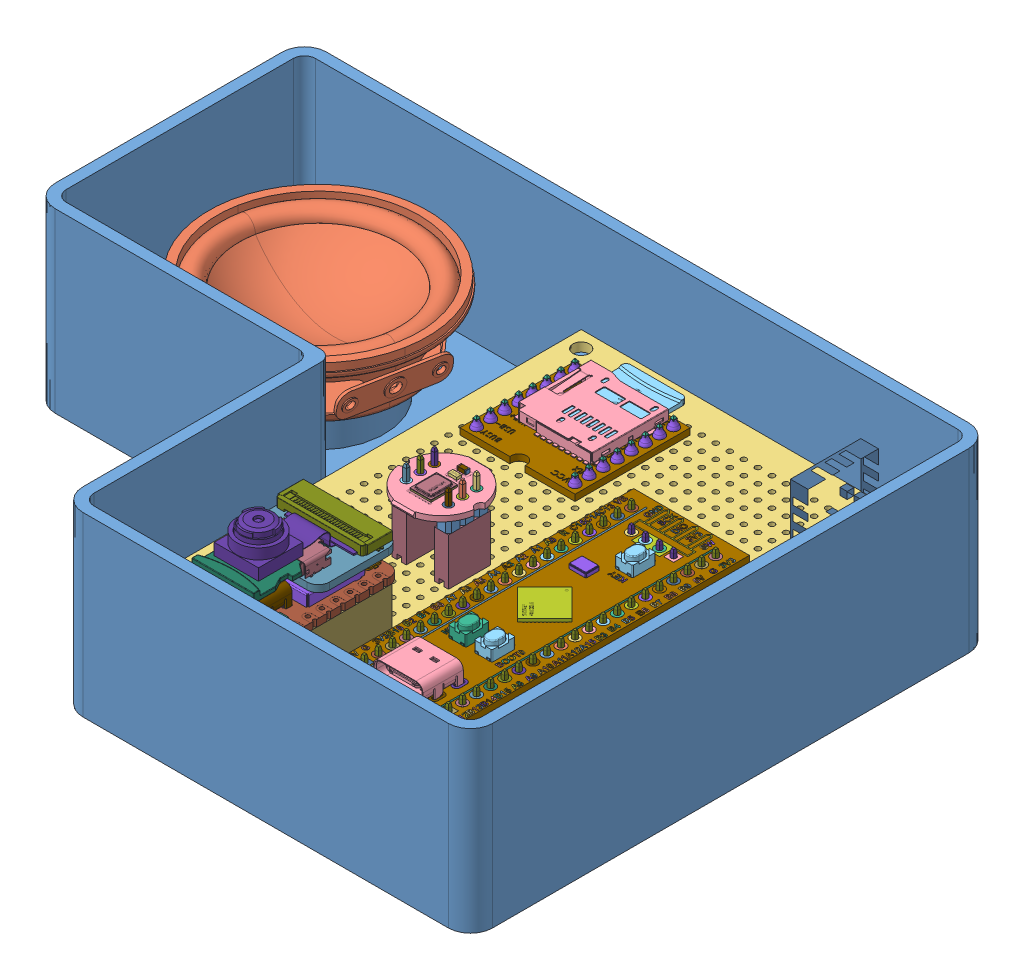
SolidWorks assembly FullLapRapVoHop, configuration Default. Lengths in mm.
Overall size (124 38.8 94).
334 component instances, 247 part files, 6 mates.
Components (placement in the parent):
- DeHop7x9-1: DeHop7x9 [Default] at (43.7132 25.4201 123.2311) size (124 32 94)
- SPEAKER 4OHM 3W.step-1: SPEAKER 4OHM 3W.step [Default] at (18.7132 43.1201 55.7311) x (-0.187693 0 0.982228) z (0.982228 0 0.187693) size (40 18.1 40)
- 3D_Final-2: 3D_Final [Default] at (43.7132 35.4201 33.2311) size (70 34.34 90)
  - BoardDong7x9-1: BoardDong7x9 [Default] at (35 1.6 45) x (0 0 -1) z (0 1 0) size (90 70 2.6)
  - blackpill v2.0 swi.STEP-1: blackpill v2.0 swi.STEP [Default] at (52.8 12.64 59.37) x (0 0 -1) z (0 1 0) size (53 20.9 10.45)
    - blackpill v2.0.step.STEP-1: blackpill v2.0.step.STEP [Default] at origin size (53 20.9 4.92)
      - USB Type C Port (SMD Type).step.STEP-1: USB Type C Port (SMD Type).step.STEP [Default] at (-19.2 0 3.305) x (0 -1 0) z (0 0 -1) size (8.94 7.9 4.2)
      - PTS810 SJK 250 SMTR LFS--3DModel-STEP-1.step.STEP-1: PTS810 SJK 250 SMTR LFS--3DModel-STEP-1.step.STEP [Default] at (14.5 -1.8498 1.7) x (1 0 0) z (0 -1 0) size (4.6 2.51 3.2)
      - PTS810 SJK 250 SMTR LFS--3DModel-STEP-1.step.STEP-2: PTS810 SJK 250 SMTR LFS--3DModel-STEP-1.step.STEP [Default] at (-11.4 -2.3498 1.7) x (1 0 0) z (0 -1 0) size (4.6 2.51 3.2)
      - PTS810 SJK 250 SMTR LFS--3DModel-STEP-1 v2(Mirror).step.STEP-1: PTS810 SJK 250 SMTR LFS--3DModel-STEP-1 v2(Mirror).step.STEP [Default] at (-11.4 2.3498 1.7) x (1 0 0) z (0 -1 0) size (4.6 2.51 3.2)
      - STM32F411CEU6.step.STEP-1: STM32F411CEU6.step.STEP [Default] at (0 0 1.7) x (-0.707107 -0.707107 0) z (-0.707107 0.707107 0) size (7 0.6 7)
      - ECS-135.60-12-33Q-JES-TR.step.STEP-1: ECS-135.60-12-33Q-JES-TR.step.STEP [Default] at (9.3867 2.3215 1.7) x (0 -1 0) z (-1 0 0) size (3.2 0.8 2.5)
      - DIY_black_pill.step.STEP-1: DIY_black_pill.step.STEP [Default] at origin size (53 20.9 1.7)
      - DIY_black_pill-0.step.STEP-1: DIY_black_pill-0.step.STEP [Default] at origin size (1.8 1.8 1.72)
      - DIY_black_pill-1.step.STEP-1: DIY_black_pill-1.step.STEP [Default] at origin size (1.8 1.8 1.72)
      - DIY_black_pill-2.step.STEP-1: DIY_black_pill-2.step.STEP [Default] at origin size (1.8 1.8 1.72)
      - DIY_black_pill-3.step.STEP-1: DIY_black_pill-3.step.STEP [Default] at origin size (1.8 1.8 1.72)
      - DIY_black_pill-4.step.STEP-1: DIY_black_pill-4.step.STEP [Default] at origin size (1.8 1.8 1.72)
      - DIY_black_pill-5.step.STEP-1: DIY_black_pill-5.step.STEP [Default] at origin size (1.8 1.8 1.72)
      - DIY_black_pill-6.step.STEP-1: DIY_black_pill-6.step.STEP [Default] at origin size (1.8 1.8 1.72)
      - DIY_black_pill-7.step.STEP-1: DIY_black_pill-7.step.STEP [Default] at origin size (1.8 1.8 1.72)
      - DIY_black_pill-8.step.STEP-1: DIY_black_pill-8.step.STEP [Default] at origin size (1.8 1.8 1.72)
      - DIY_black_pill-9.step.STEP-1: DIY_black_pill-9.step.STEP [Default] at origin size (1.8 1.8 1.72)
      - DIY_black_pill-10.step.STEP-1: DIY_black_pill-10.step.STEP [Default] at origin size (1.8 1.8 1.72)
      - DIY_black_pill-11.step.STEP-1: DIY_black_pill-11.step.STEP [Default] at origin size (1.8 1.8 1.72)
      - DIY_black_pill-12.step.STEP-1: DIY_black_pill-12.step.STEP [Default] at origin size (1.8 1.8 1.72)
      - DIY_black_pill-13.step.STEP-1: DIY_black_pill-13.step.STEP [Default] at origin size (1.8 1.8 1.72)
      - DIY_black_pill-14.step.STEP-1: DIY_black_pill-14.step.STEP [Default] at origin size (1.8 1.8 1.72)
      - DIY_black_pill-15.step.STEP-1: DIY_black_pill-15.step.STEP [Default] at origin size (1.8 1.8 1.72)
      - DIY_black_pill-16.step.STEP-1: DIY_black_pill-16.step.STEP [Default] at origin size (1.8 1.8 1.72)
      - DIY_black_pill-17.step.STEP-1: DIY_black_pill-17.step.STEP [Default] at origin size (1.8 1.8 1.72)
      - DIY_black_pill-18.step.STEP-1: DIY_black_pill-18.step.STEP [Default] at origin size (1.8 1.8 1.72)
      - DIY_black_pill-19.step.STEP-1: DIY_black_pill-19.step.STEP [Default] at origin size (1.8 1.8 1.72)
      - DIY_black_pill-20.step.STEP-1: DIY_black_pill-20.step.STEP [Default] at origin size (1.8 1.8 1.72)
      - DIY_black_pill-21.step.STEP-1: DIY_black_pill-21.step.STEP [Default] at origin size (1.8 1.8 1.72)
      - DIY_black_pill-22.step.STEP-1: DIY_black_pill-22.step.STEP [Default] at origin size (1.8 1.8 1.72)
      - DIY_black_pill-23.step.STEP-1: DIY_black_pill-23.step.STEP [Default] at origin size (1.8 1.8 1.72)
      - DIY_black_pill-24.step.STEP-1: DIY_black_pill-24.step.STEP [Default] at origin size (1.8 1.8 1.72)
      - DIY_black_pill-25.step.STEP-1: DIY_black_pill-25.step.STEP [Default] at origin size (1.8 1.8 1.72)
      - DIY_black_pill-26.step.STEP-1: DIY_black_pill-26.step.STEP [Default] at origin size (1.8 1.8 1.72)
      - DIY_black_pill-27.step.STEP-1: DIY_black_pill-27.step.STEP [Default] at origin size (1.8 1.8 1.72)
      - DIY_black_pill-28.step.STEP-1: DIY_black_pill-28.step.STEP [Default] at origin size (1.8 1.8 1.72)
      - DIY_black_pill-29.step.STEP-1: DIY_black_pill-29.step.STEP [Default] at origin size (1.8 1.8 1.72)
      - DIY_black_pill-30.step.STEP-1: DIY_black_pill-30.step.STEP [Default] at origin size (1.8 1.8 1.72)
      - DIY_black_pill-31.step.STEP-1: DIY_black_pill-31.step.STEP [Default] at origin size (1.8 1.8 1.72)
      - DIY_black_pill-32.step.STEP-1: DIY_black_pill-32.step.STEP [Default] at origin size (1.8 1.8 1.72)
      - DIY_black_pill-33.step.STEP-1: DIY_black_pill-33.step.STEP [Default] at origin size (1.8 1.8 1.72)
      - DIY_black_pill-34.step.STEP-1: DIY_black_pill-34.step.STEP [Default] at origin size (1.8 1.8 1.72)
      - DIY_black_pill-35.step.STEP-1: DIY_black_pill-35.step.STEP [Default] at origin size (1.8 1.8 1.72)
      - DIY_black_pill-36.step.STEP-1: DIY_black_pill-36.step.STEP [Default] at origin size (1.8 1.8 1.72)
      - DIY_black_pill-37.step.STEP-1: DIY_black_pill-37.step.STEP [Default] at origin size (1.8 1.8 1.72)
      - DIY_black_pill-38.step.STEP-1: DIY_black_pill-38.step.STEP [Default] at origin size (1.8 1.8 1.72)
      - DIY_black_pill-39.step.STEP-1: DIY_black_pill-39.step.STEP [Default] at origin size (1.8 1.8 1.72)
      - DIY_black_pill-40.step.STEP-1: DIY_black_pill-40.step.STEP [Default] at origin size (51.2 0.3 0.01)
      - DIY_black_pill-41.step.STEP-1: DIY_black_pill-41.step.STEP [Default] at origin size (51.2 0.3 0.01)
      - DIY_black_pill-42.step.STEP-1: DIY_black_pill-42.step.STEP [Default] at origin size (0.93 1 0.01)
      - DIY_black_pill-43.step.STEP-1: DIY_black_pill-43.step.STEP [Default] at origin size (0.94 1.03 0.01)
      - DIY_black_pill-44.step.STEP-1: DIY_black_pill-44.step.STEP [Default] at origin size (0.93 1 0.01)
      - DIY_black_pill-45.step.STEP-1: DIY_black_pill-45.step.STEP [Default] at origin size (0.67 1.02 0.01)
      - DIY_black_pill-46.step.STEP-1: DIY_black_pill-46.step.STEP [Default] at origin size (0.66 1.02 0.01)
      - DIY_black_pill-47.step.STEP-1: DIY_black_pill-47.step.STEP [Default] at origin size (0.84 1 0.01)
      - DIY_black_pill-48.step.STEP-1: DIY_black_pill-48.step.STEP [Default] at origin size (0.67 1.02 0.01)
      - DIY_black_pill-49.step.STEP-1: DIY_black_pill-49.step.STEP [Default] at origin size (0.84 1.01 0.01)
      - DIY_black_pill-50.step.STEP-1: DIY_black_pill-50.step.STEP [Default] at origin size (0.72 1.01 0.01)
      - DIY_black_pill-51.step.STEP-1: DIY_black_pill-51.step.STEP [Default] at origin size (0.84 1 0.01)
      - DIY_black_pill-52.step.STEP-1: DIY_black_pill-52.step.STEP [Default] at origin size (0.67 1 0.01)
      - DIY_black_pill-53.step.STEP-1: DIY_black_pill-53.step.STEP [Default] at origin size (1 1 0.01)
      - DIY_black_pill-54.step.STEP-1: DIY_black_pill-54.step.STEP [Default] at origin size (0.44 1 0.01)
      - DIY_black_pill-55.step.STEP-1: DIY_black_pill-55.step.STEP [Default] at origin size (0.44 1 0.01)
      - DIY_black_pill-56.step.STEP-1: DIY_black_pill-56.step.STEP [Default] at origin size (1 1 0.01)
      - DIY_black_pill-57.step.STEP-1: DIY_black_pill-57.step.STEP [Default] at origin size (0.44 1 0.01)
      - DIY_black_pill-58.step.STEP-1: DIY_black_pill-58.step.STEP [Default] at origin size (0.67 1.02 0.01)
      - DIY_black_pill-59.step.STEP-1: DIY_black_pill-59.step.STEP [Default] at origin size (0.66 1.02 0.01)
      - DIY_black_pill-60.step.STEP-1: DIY_black_pill-60.step.STEP [Default] at origin size (0.67 1 0.01)
      - DIY_black_pill-61.step.STEP-1: DIY_black_pill-61.step.STEP [Default] at origin size (0.84 1 0.01)
      - DIY_black_pill-62.step.STEP-1: DIY_black_pill-62.step.STEP [Default] at origin size (0.44 1 0.01)
      - DIY_black_pill-63.step.STEP-1: DIY_black_pill-63.step.STEP [Default] at origin size (0.66 1.02 0.01)
      - DIY_black_pill-64.step.STEP-1: DIY_black_pill-64.step.STEP [Default] at origin size (0.44 1 0.01)
      - DIY_black_pill-65.step.STEP-1: DIY_black_pill-65.step.STEP [Default] at origin size (0.84 1 0.01)
      - DIY_black_pill-66.step.STEP-1: DIY_black_pill-66.step.STEP [Default] at origin size (0.72 1 0.01)
      - DIY_black_pill-67.step.STEP-1: DIY_black_pill-67.step.STEP [Default] at origin size (0.44 1 0.01)
      - DIY_black_pill-68.step.STEP-1: DIY_black_pill-68.step.STEP [Default] at origin size (0.84 1 0.01)
      - DIY_black_pill-69.step.STEP-1: DIY_black_pill-69.step.STEP [Default] at origin size (1 1 0.01)
      - DIY_black_pill-70.step.STEP-1: DIY_black_pill-70.step.STEP [Default] at origin size (1 1 0.01)
      - DIY_black_pill-71.step.STEP-1: DIY_black_pill-71.step.STEP [Default] at origin size (0.65 1.02 0.01)
      - DIY_black_pill-72.step.STEP-1: DIY_black_pill-72.step.STEP [Default] at origin size (0.44 1 0.01)
      - DIY_black_pill-73.step.STEP-1: DIY_black_pill-73.step.STEP [Default] at origin size (1 1 0.01)
      - DIY_black_pill-74.step.STEP-1: DIY_black_pill-74.step.STEP [Default] at origin size (0.67 1 0.01)
      - DIY_black_pill-75.step.STEP-1: DIY_black_pill-75.step.STEP [Default] at origin size (0.44 1 0.01)
      - DIY_black_pill-76.step.STEP-1: DIY_black_pill-76.step.STEP [Default] at origin size (1 1 0.01)
      - DIY_black_pill-77.step.STEP-1: DIY_black_pill-77.step.STEP [Default] at origin size (0.66 1.02 0.01)
      - DIY_black_pill-78.step.STEP-1: DIY_black_pill-78.step.STEP [Default] at origin size (0.84 1.01 0.01)
      - DIY_black_pill-79.step.STEP-1: DIY_black_pill-79.step.STEP [Default] at origin size (0.67 1.01 0.01)
      - DIY_black_pill-80.step.STEP-1: DIY_black_pill-80.step.STEP [Default] at origin size (0.84 1 0.01)
      - DIY_black_pill-81.step.STEP-1: DIY_black_pill-81.step.STEP [Default] at origin size (0.66 0.99 0.01)
      - DIY_black_pill-82.step.STEP-1: DIY_black_pill-82.step.STEP [Default] at origin size (0.84 1 0.01)
      - DIY_black_pill-83.step.STEP-1: DIY_black_pill-83.step.STEP [Default] at origin size (0.84 1 0.01)
      - DIY_black_pill-84.step.STEP-1: DIY_black_pill-84.step.STEP [Default] at origin size (0.67 1 0.01)
      - DIY_black_pill-85.step.STEP-1: DIY_black_pill-85.step.STEP [Default] at origin size (0.66 1.02 0.01)
      - DIY_black_pill-86.step.STEP-1: DIY_black_pill-86.step.STEP [Default] at origin size (0.66 1.02 0.01)
      - DIY_black_pill-87.step.STEP-1: DIY_black_pill-87.step.STEP [Default] at origin size (0.67 1 0.01)
      - DIY_black_pill-88.step.STEP-1: DIY_black_pill-88.step.STEP [Default] at origin size (0.44 1 0.01)
      - DIY_black_pill-89.step.STEP-1: DIY_black_pill-89.step.STEP [Default] at origin size (0.84 1 0.01)
      - DIY_black_pill-90.step.STEP-1: DIY_black_pill-90.step.STEP [Default] at origin size (1 1 0.01)
      - DIY_black_pill-91.step.STEP-1: DIY_black_pill-91.step.STEP [Default] at origin size (0.84 1 0.01)
      - DIY_black_pill-92.step.STEP-1: DIY_black_pill-92.step.STEP [Default] at origin size (0.44 1 0.01)
      - DIY_black_pill-93.step.STEP-1: DIY_black_pill-93.step.STEP [Default] at origin size (0.87 1.03 0.01)
      - DIY_black_pill-94.step.STEP-1: DIY_black_pill-94.step.STEP [Default] at origin size (0.44 1 0.01)
      - DIY_black_pill-95.step.STEP-1: DIY_black_pill-95.step.STEP [Default] at origin size (0.44 1 0.01)
      - DIY_black_pill-96.step.STEP-1: DIY_black_pill-96.step.STEP [Default] at origin size (0.9 1 0.01)
      - DIY_black_pill-97.step.STEP-1: DIY_black_pill-97.step.STEP [Default] at origin size (0.65 1.02 0.01)
      - DIY_black_pill-98.step.STEP-1: DIY_black_pill-98.step.STEP [Default] at origin size (1 1 0.01)
      - DIY_black_pill-99.step.STEP-1: DIY_black_pill-99.step.STEP [Default] at origin size (0.72 1 0.01)
      - DIY_black_pill-100.step.STEP-1: DIY_black_pill-100.step.STEP [Default] at origin size (1 1 0.01)
      - DIY_black_pill-101.step.STEP-1: DIY_black_pill-101.step.STEP [Default] at origin size (0.67 1.02 0.01)
      - DIY_black_pill-102.step.STEP-1: DIY_black_pill-102.step.STEP [Default] at origin size (0.65 1.02 0.01)
      - DIY_black_pill-103.step.STEP-1: DIY_black_pill-103.step.STEP [Default] at origin size (1 1 0.01)
      - DIY_black_pill-104.step.STEP-1: DIY_black_pill-104.step.STEP [Default] at origin size (0.84 1 0.01)
      - DIY_black_pill-105.step.STEP-1: DIY_black_pill-105.step.STEP [Default] at origin size (0.84 1 0.01)
      - DIY_black_pill-106.step.STEP-1: DIY_black_pill-106.step.STEP [Default] at origin size (0.65 1.02 0.01)
      - DIY_black_pill-107.step.STEP-1: DIY_black_pill-107.step.STEP [Default] at origin size (0.66 1.02 0.01)
      - DIY_black_pill-108.step.STEP-1: DIY_black_pill-108.step.STEP [Default] at origin size (0.66 1.02 0.01)
      - DIY_black_pill-109.step.STEP-1: DIY_black_pill-109.step.STEP [Default] at origin size (0.67 1 0.01)
      - DIY_black_pill-110.step.STEP-1: DIY_black_pill-110.step.STEP [Default] at origin size (0.93 1 0.01)
      - DIY_black_pill-111.step.STEP-1: DIY_black_pill-111.step.STEP [Default] at origin size (0.94 1.03 0.01)
      - DIY_black_pill-112.step.STEP-1: DIY_black_pill-112.step.STEP [Default] at origin size (0.93 1 0.01)
      - DIY_black_pill-113.step.STEP-1: DIY_black_pill-113.step.STEP [Default] at origin size (0.44 1 0.01)
      - DIY_black_pill-114.step.STEP-1: DIY_black_pill-114.step.STEP [Default] at origin size (0.84 1 0.01)
      - DIY_black_pill-115.step.STEP-1: DIY_black_pill-115.step.STEP [Default] at origin size (0.67 1 0.01)
      - DIY_black_pill-116.step.STEP-1: DIY_black_pill-116.step.STEP [Default] at origin size (0.44 1 0.01)
      - DIY_black_pill-117.step.STEP-1: DIY_black_pill-117.step.STEP [Default] at origin size (0.66 0.99 0.01)
      - DIY_black_pill-118.step.STEP-1: DIY_black_pill-118.step.STEP [Default] at origin size (0.84 1 0.01)
      - DIY_black_pill-119.step.STEP-1: DIY_black_pill-119.step.STEP [Default] at origin size (1 1 0.01)
      - DIY_black_pill-120.step.STEP-1: DIY_black_pill-120.step.STEP [Default] at origin size (0.67 1 0.01)
      - DIY_black_pill-121.step.STEP-1: DIY_black_pill-121.step.STEP [Default] at origin size (1 1 0.01)
      - DIY_black_pill-122.step.STEP-1: DIY_black_pill-122.step.STEP [Default] at origin size (0.66 1.02 0.01)
      - DIY_black_pill-123.step.STEP-1: DIY_black_pill-123.step.STEP [Default] at origin size (1 1 0.01)
      - DIY_black_pill-124.step.STEP-1: DIY_black_pill-124.step.STEP [Default] at origin size (0.67 1 0.01)
      - DIY_black_pill-125.step.STEP-1: DIY_black_pill-125.step.STEP [Default] at origin size (0.87 1.03 0.01)
      - DIY_black_pill-126.step.STEP-1: DIY_black_pill-126.step.STEP [Default] at origin size (0.72 1 0.01)
      - DIY_black_pill-127.step.STEP-1: DIY_black_pill-127.step.STEP [Default] at origin size (0.66 1.02 0.01)
      - DIY_black_pill-128.step.STEP-1: DIY_black_pill-128.step.STEP [Default] at origin size (0.87 1.03 0.01)
      - DIY_black_pill-129.step.STEP-1: DIY_black_pill-129.step.STEP [Default] at origin size (0.93 1 0.01)
      - DIY_black_pill-130.step.STEP-1: DIY_black_pill-130.step.STEP [Default] at origin size (0.44 1 0.01)
      - DIY_black_pill-131.step.STEP-1: DIY_black_pill-131.step.STEP [Default] at origin size (2.55 1.5 1.72)
      - DIY_black_pill-132.step.STEP-1: DIY_black_pill-132.step.STEP [Default] at origin size (2.6 1.5 1.72)
      - DIY_black_pill-133.step.STEP-1: DIY_black_pill-133.step.STEP [Default] at origin size (2.55 1.5 1.72)
      - DIY_black_pill-134.step.STEP-1: DIY_black_pill-134.step.STEP [Default] at origin size (2.6 1.5 1.72)
      - DIY_black_pill-135.step.STEP-1: DIY_black_pill-135.step.STEP [Default] at origin size (1 1 0.01)
      - DIY_black_pill-136.step.STEP-1: DIY_black_pill-136.step.STEP [Default] at origin size (0.67 1.01 0.01)
      - DIY_black_pill-137.step.STEP-1: DIY_black_pill-137.step.STEP [Default] at origin size (1.8 1.8 1.72)
      - DIY_black_pill-138.step.STEP-1: DIY_black_pill-138.step.STEP [Default] at origin size (1.8 1.8 1.72)
      - DIY_black_pill-139.step.STEP-1: DIY_black_pill-139.step.STEP [Default] at origin size (1.8 1.8 1.72)
      - DIY_black_pill-140.step.STEP-1: DIY_black_pill-140.step.STEP [Default] at origin size (1.8 1.8 1.72)
      - DIY_black_pill-141.step.STEP-1: DIY_black_pill-141.step.STEP [Default] at origin size (8.17 10.16 0.01)
      - DIY_black_pill-142.step.STEP-1: DIY_black_pill-142.step.STEP [Default] at origin size (1.31 1 0.01)
      - DIY_black_pill-143.step.STEP-1: DIY_black_pill-143.step.STEP [Default] at origin size (0.93 1 0.01)
      - DIY_black_pill-144.step.STEP-1: DIY_black_pill-144.step.STEP [Default] at origin size (0.84 1 0.01)
      - DIY_black_pill-145.step.STEP-1: DIY_black_pill-145.step.STEP [Default] at origin size (0.2 1 0.01)
      - DIY_black_pill-146.step.STEP-1: DIY_black_pill-146.step.STEP [Default] at origin size (0.87 1.03 0.01)
      - DIY_black_pill-147.step.STEP-1: DIY_black_pill-147.step.STEP [Default] at origin size (0.94 1.03 0.01)
      - DIY_black_pill-148.step.STEP-1: DIY_black_pill-148.step.STEP [Default] at origin size (0.79 1 0.01)
      - DIY_black_pill-149.step.STEP-1: DIY_black_pill-149.step.STEP [Default] at origin size (0.84 1 0.01)
      - DIY_black_pill-150.step.STEP-1: DIY_black_pill-150.step.STEP [Default] at origin size (0.9 1 0.01)
      - DIY_black_pill-151.step.STEP-1: DIY_black_pill-151.step.STEP [Default] at origin size (0.81 1.03 0.01)
      - DIY_black_pill-152.step.STEP-1: DIY_black_pill-152.step.STEP [Default] at origin size (0.97 1.03 0.01)
      - DIY_black_pill-153.step.STEP-1: DIY_black_pill-153.step.STEP [Default] at origin size (0.66 1.02 0.01)
      - DIY_black_pill-154.step.STEP-1: DIY_black_pill-154.step.STEP [Default] at origin size (0.66 1.02 0.01)
      - DIY_black_pill-155.step.STEP-1: DIY_black_pill-155.step.STEP [Default] at origin size (0.81 1.03 0.01)
      - DIY_black_pill-156.step.STEP-1: DIY_black_pill-156.step.STEP [Default] at origin size (0.9 1 0.01)
      - DIY_black_pill-157.step.STEP-1: DIY_black_pill-157.step.STEP [Default] at origin size (0.81 1.03 0.01)
      - DIY_black_pill-158.step.STEP-1: DIY_black_pill-158.step.STEP [Default] at origin size (0.97 1.03 0.01)
      - DIY_black_pill-159.step.STEP-1: DIY_black_pill-159.step.STEP [Default] at origin size (0.97 1.03 0.01)
      - DIY_black_pill-160.step.STEP-1: DIY_black_pill-160.step.STEP [Default] at origin size (1.01 0.91 0.01)
      - DIY_black_pill-161.step.STEP-1: DIY_black_pill-161.step.STEP [Default] at origin size (1 0.94 0.01)
      - DIY_black_pill-162.step.STEP-1: DIY_black_pill-162.step.STEP [Default] at origin size (1 0.77 0.01)
      - DIY_black_pill-163.step.STEP-1: DIY_black_pill-163.step.STEP [Default] at origin size (0.79 1 0.01)
      - DIY_black_pill-164.step.STEP-1: DIY_black_pill-164.step.STEP [Default] at origin size (0.65 1.02 0.01)
      - DIY_black_pill-165.step.STEP-1: DIY_black_pill-165.step.STEP [Default] at origin size (0.84 1 0.01)
      - DIY_black_pill-166.step.STEP-1: DIY_black_pill-166.step.STEP [Default] at origin size (0.79 1 0.01)
      - DIY_black_pill-167.step.STEP-1: DIY_black_pill-167.step.STEP [Default] at origin size (0.79 1 0.01)
    - 1x20 Male Pin Header.STEP-1: 1x20 Male Pin Header.STEP [Default] at (23.26 -7.6 0) x (-1 0 0) z (0 -1 0) size (50.8 8.54 2.5)
    - 1x20 Male Pin Header.STEP-2: 1x20 Male Pin Header.STEP [Default] at (23.26 7.6 0) x (-1 0 0) z (0 -1 0) size (50.8 8.54 2.5)
    - 1x4 Male Pin Header.STEP-1: 1x4 Male Pin Header.STEP [Default] at (19.45 -3.81 0) x (0 1 0) z (-1 0 0) size (10.17 8.54 2.5)
  - Seeed Studio XIAO-ESP32-S3-Sense-1: Seeed Studio XIAO-ESP32-S3-Sense [Default] at (16.1886 10.35 72.4693) x (0 0 1) z (-1 0 0) size (24.36 13.98 17.79)
    - Seeed Studio XIAO-ESP32-S3-Sense.step-1: Seeed Studio XIAO-ESP32-S3-Sense.step [Default] at origin size (24.36 13.98 17.79)
      - Seeed Studio XIAO-ESP32-S3 (Sense).step-1: Seeed Studio XIAO-ESP32-S3 (Sense).step [Default] at origin size (22.49 4.48 17.79)
        - USB TYPE C PORT.step-1: USB TYPE C PORT.step [Default] at (4.3161 13.395 -12.1571) x (0 0 -1) z (0 -1 0) size (8.94 7.9 4.2)
          - USB TYPE C PORT (1).step-1: USB TYPE C PORT (1).step [Default] at (-3.0192 1.0963 5.395) size (8.94 7.9 4.2)
            - BOSS-EXTRUDE14_8_.step-1: BOSS-EXTRUDE14_8_.step [Default] at (-3.0192 1.0963 5.395) size (0.6 1 0.3)
            - BOSS-EXTRUDE7_4_.step-1: BOSS-EXTRUDE7_4_.step [Default] at (-3.0192 1.0963 5.395) size (0.3 3.78 0.75)
            - BOSS-EXTRUDE7_3_.step-1: BOSS-EXTRUDE7_3_.step [Default] at (-3.0192 1.0963 5.395) size (0.3 3.78 0.75)
            - BOSS-EXTRUDE14_4_.step-1: BOSS-EXTRUDE14_4_.step [Default] at (-3.0192 1.0963 5.395) size (0.3 1 0.3)
            - BOSS-EXTRUDE14_2_.step-1: BOSS-EXTRUDE14_2_.step [Default] at (-3.0192 1.0963 5.395) size (0.6 1 0.3)
            - BOSS-EXTRUDE14_11_.step-1: BOSS-EXTRUDE14_11_.step [Default] at (-3.0192 1.0963 5.395) size (0.3 1 0.3)
            - BOSS-EXTRUDE7_7_.step-1: BOSS-EXTRUDE7_7_.step [Default] at (-3.0192 1.0963 5.395) size (0.3 3.78 0.75)
            - BOSS-EXTRUDE14_9_.step-1: BOSS-EXTRUDE14_9_.step [Default] at (-3.0192 1.0963 5.395) size (0.3 1 0.3)
            - BOSS-EXTRUDE14_3_.step-1: BOSS-EXTRUDE14_3_.step [Default] at (-3.0192 1.0963 5.395) size (0.3 1 0.3)
            - BOSS-EXTRUDE14_7_.step-1: BOSS-EXTRUDE14_7_.step [Default] at (-3.0192 1.0963 5.395) size (0.6 1 0.3)
            - MIRROR2.step-1: MIRROR2.step [Default] at (-3.0192 1.0963 5.395) size (6.7 4.6 0.7)
            - BOSS-EXTRUDE14_5_.step-1: BOSS-EXTRUDE14_5_.step [Default] at (-3.0192 1.0963 5.395) size (0.3 1 0.3)
            - BOSS-EXTRUDE14_12_.step-1: BOSS-EXTRUDE14_12_.step [Default] at (-3.0192 1.0963 5.395) size (0.3 1 0.3)
            - BOSS-EXTRUDE7_8_.step-1: BOSS-EXTRUDE7_8_.step [Default] at (-3.0192 1.0963 5.395) size (0.3 3.78 0.75)
            - BOSS-EXTRUDE7_1_.step-1: BOSS-EXTRUDE7_1_.step [Default] at (-3.0192 1.0963 5.395) size (0.3 3.78 0.75)
            - BOSS-EXTRUDE14_10_.step-1: BOSS-EXTRUDE14_10_.step [Default] at (-3.0192 1.0963 5.395) size (0.3 1 0.3)
            - BOSS-EXTRUDE7_9_.step-1: BOSS-EXTRUDE7_9_.step [Default] at (-3.0192 1.0963 5.395) size (0.3 3.78 0.75)
            - BOSS-EXTRUDE14_6_.step-1: BOSS-EXTRUDE14_6_.step [Default] at (-3.0192 1.0963 5.395) size (0.6 1 0.3)
            - CHAMFER9.step-1: CHAMFER9.step [Default] at (-3.0192 1.0963 5.395) size (8.94 7.3 4.2)
            - BOSS-EXTRUDE14_1_.step-1: BOSS-EXTRUDE14_1_.step [Default] at (-3.0192 1.0963 5.395) size (0.3 1 0.3)
            - BOSS-EXTRUDE7_6_.step-1: BOSS-EXTRUDE7_6_.step [Default] at (-3.0192 1.0963 5.395) size (0.3 3.78 0.75)
            - BOSS-EXTRUDE7_2_.step-1: BOSS-EXTRUDE7_2_.step [Default] at (-3.0192 1.0963 5.395) size (0.3 3.78 0.75)
            - CUT-EXTRUDE5.step-1: CUT-EXTRUDE5.step [Default] at (-3.0192 1.0963 5.395) size (8.54 2 3.59)
            - BOSS-EXTRUDE7_5_.step-1: BOSS-EXTRUDE7_5_.step [Default] at (-3.0192 1.0963 5.395) size (0.3 3.78 0.75)
        - SKTAAAE010 v1.step-1: SKTAAAE010 v1.step [Default] at (10.7092 1 -12.0449) x (1 0 0) z (0 1 0) size (3.09 1.6 0.73)
          - Body.step-1: Body.step [Default] at (0 0 0.1) size (2.6 1.6 0.63)
          - Pins.step-1: Pins.step [Default] at origin size (3.09 1.19 0.1)
        - SKTAAAE010 v1.step-2: SKTAAAE010 v1.step [Default] at (10.6911 1 -0.1868) x (1 0 0) z (0 1 0) size (3.09 1.6 0.73)
          - Body.step-1: Body.step [Default] at (0 0 0.1) size (2.6 1.6 0.63)
          - Pins.step-1: Pins.step [Default] at origin size (3.09 1.19 0.1)
        - Shield.step-1: Shield.step [Default] at origin size (10.6 2.7 12.6)
        - U.FL-R-SMT-1_10_ v1.step-1: U.FL-R-SMT-1_10_ v1.step [Default] at (-6.9517 1 -10.8381) x (1 0 0) z (0 1 0) size (3 3.1 1.25)
        - DF40C-30DP-0.4V_51_ v1.step-1: DF40C-30DP-0.4V_51_ v1.step [Default] at (-6.0667 1.65 -7.7227) size (2.97 1.14 7.52)
        - Seeed Studio XIAO-ESP32-S3 (Sense)-0.step-1: Seeed Studio XIAO-ESP32-S3 (Sense)-0.step [Default] at origin size (20.97 1.28 17.79)
      - Sense Expansion Board.step-1: Sense Expansion Board.step [Default] at (-0.3 4.5 0) x (-1 0 0) z (0 0 1) size (24.36 7.23 16.78)
        - DF40HC(3.0)-30DS.step-1: DF40HC(3.0)-30DS.step [Default] at (6.4217 1.57 -3.0777) x (-1 0 0) z (0 0 1) size (3.38 2.9 8.6)
        - 10067099-200LF v1.step-1: 10067099-200LF v1.step [Default] at (-1.3077 -2.08 -6.0846) x (0 0 -1) z (-1 0 0) size (11.4 2.65 5.5)
        - PCB.step-1: PCB.step [Default] at origin size (14.68 1.25 16.78)
        - MicroSD v2.step-1: MicroSD v2.step [Default] at (-8.16 -2.1 -6.9267) x (1 0 0) z (0 0 -1) size (15.06 1.66 11.19)
        - JUSHUO AFC01-S24FCA-00.step-1: JUSHUO AFC01-S24FCA-00.step [Default] at (6.9932 -0.67 -6.0797) x (0 0 1) z (0 -1 0) size (16.2 6.01 2.01)
      - Camer Module.step-1: Camer Module.step [Default] at (-7.2 6 -13) size (19.95 8.11 12.5)
  - INMP441 I2S Microphone Module v15-1: INMP441 I2S Microphone Module v15 [Default] at (23.57 12.61 48.81) size (13.77 11.25 14.24)
    - INMP441 I2S Microphone Module v15.step-1: INMP441 I2S Microphone Module v15.step [Default] at origin size (13.77 11.25 14.24)
      - C0603_070.step-1: C0603_070.step [Default] at (0 8.5 0) x (1 0 0) z (0 1 0) size (1.6 0.8 0.7)
        - C0603_070_1.step-1: C0603_070_1.step [Default] at origin size (1.6 0.8 0.7)
          - Part 3.step-1: Part 3.step [Default] at (0 4 -7.535) size (1.4 0.77 0.67)
          - Part 2.step-1: Part 2.step [Default] at (0 4 -7.535) size (0.2 0.8 0.7)
          - Part 1.step-1: Part 1.step [Default] at (0 4 -7.535) size (0.2 0.8 0.7)
      - 0603 Resistor.step-1: 0603 Resistor.step [Default] at (0 0.98 -2.4) x (1 0 0) z (0 1 0) size (1.6 0.9 0.5)
      - INMP441 I2S Microphone Module.step-1: INMP441 I2S Microphone Module.step [Default] at origin size (13.77 1 14.24)
      - INMP441 I2S Microphone Module-0.step-1: INMP441 I2S Microphone Module-0.step [Default] at origin size (1.6 1 1.6)
      - INMP441 I2S Microphone Module-1.step-1: INMP441 I2S Microphone Module-1.step [Default] at origin size (1.6 1 1.6)
      - INMP441 I2S Microphone Module-2.step-1: INMP441 I2S Microphone Module-2.step [Default] at origin size (1.6 1 1.6)
      - INMP441 I2S Microphone Module-3.step-1: INMP441 I2S Microphone Module-3.step [Default] at origin size (1.6 1 1.6)
      - INMP441 I2S Microphone Module-4.step-1: INMP441 I2S Microphone Module-4.step [Default] at origin size (1.6 1 1.6)
      - INMP441 I2S Microphone Module-5.step-1: INMP441 I2S Microphone Module-5.step [Default] at origin size (1.6 1 1.6)
      - INMP441 I2S Microphone Module-6.step-1: INMP441 I2S Microphone Module-6.step [Default] at origin size (1.6 1 1.6)
      - INMP441 I2S Microphone Module-7.step-1: INMP441 I2S Microphone Module-7.step [Default] at origin size (3.79 0.3 4.79)
      - INMP441 I2S Microphone Module-8.step-1: INMP441 I2S Microphone Module-8.step [Default] at origin size (3.79 0.41 4.79)
      - INMP441 I2S Microphone Module-9.step-1: INMP441 I2S Microphone Module-9.step [Default] at origin size (0.65 11.25 0.65)
      - INMP441 I2S Microphone Module-10.step-1: INMP441 I2S Microphone Module-10.step [Default] at origin size (2.55 2.5 7.63)
      - INMP441 I2S Microphone Module-11.step-1: INMP441 I2S Microphone Module-11.step [Default] at origin size (0.65 11.25 0.65)
      - INMP441 I2S Microphone Module-12.step-1: INMP441 I2S Microphone Module-12.step [Default] at origin size (0.65 11.25 0.65)
      - INMP441 I2S Microphone Module-13.step-1: INMP441 I2S Microphone Module-13.step [Default] at origin size (0.65 11.25 0.65)
      - INMP441 I2S Microphone Module-14.step-1: INMP441 I2S Microphone Module-14.step [Default] at origin size (2.55 2.5 7.63)
      - INMP441 I2S Microphone Module-15.step-1: INMP441 I2S Microphone Module-15.step [Default] at origin size (0.65 11.25 0.65)
      - INMP441 I2S Microphone Module-16.step-1: INMP441 I2S Microphone Module-16.step [Default] at origin size (0.65 11.25 0.65)
  - DFPlayer Mini Assem v1.step-1: DFPlayer Mini Assem v1.step [Default] at (15.95 1.6 17.06) x (-1 0 0) z (0 0 -1) size (20.8 11.2 23.46)
    - SD card Assem^DFPlayer Mini Assem v1.step-1: SD card Assem^DFPlayer Mini Assem v1.step [Default] at (-198.0203 122.5536 -43.8714) x (0 1 0) z (1 0 0) size (2.44 17.9 16) (virtual)
      - CD card slot^SD card Assem_DFPlayer Mini Assem v1.step-1: CD card slot^SD card Assem_DFPlayer Mini Assem v1.step [Default] at (-120.5536 47.0914 197.6703) x (0 0 1) z (1 0 0) size (16 15 2.44) (virtual)
      - Micro sd card^SD card Assem_DFPlayer Mini Assem v1.step-1: Micro sd card^SD card Assem_DFPlayer Mini Assem v1.step [Default] at (-120.5536 45.5089 151.9853) x (0 0 1) z (1 0 0) size (11 15 0.95) (virtual)
    - DFPlayer Mini Pin.step-1: DFPlayer Mini Pin.step [Default] at (8.89 0 8.89) x (0 0 -1) z (0 -1 0) size (2.54 2.54 11.2)
      - 11_20mm pin.step-1: 11_20mm pin.step [Default] at (0 0 2.6) size (0.63 0.63 11.2)
      - Pin Header 1x12 TH Pitch 2.step-1: Pin Header 1x12 TH Pitch 2.step [Default] at (-27.94 0 -0.0014) size (2.54 2.54 2.8)
      - solder.step-1: solder.step [Default] at (0 0 -1.15) x (1 0 0) z (0 1 0) size (1.8 1.45 1.8)
    - DFPlayer Mini Pin.step-2: DFPlayer Mini Pin.step [Default] at (-8.89 0 8.89) x (0 0 1) z (0 -1 0) size (2.54 2.54 11.2)
      - 11_20mm pin.step-1: 11_20mm pin.step [Default] at (0 0 2.6) size (0.63 0.63 11.2)
      - Pin Header 1x12 TH Pitch 2.step-1: Pin Header 1x12 TH Pitch 2.step [Default] at (-27.94 0 -0.0014) size (2.54 2.54 2.8)
      - solder.step-1: solder.step [Default] at (0 0 -1.15) x (1 0 0) z (0 1 0) size (1.8 1.45 1.8)
    - DFPlayer Mini Pin.step-3: DFPlayer Mini Pin.step [Default] at (-8.89 0 6.35) x (0 0 1) z (0 -1 0) size (2.54 2.54 11.2)
      - 11_20mm pin.step-1: 11_20mm pin.step [Default] at (0 0 2.6) size (0.63 0.63 11.2)
      - Pin Header 1x12 TH Pitch 2.step-1: Pin Header 1x12 TH Pitch 2.step [Default] at (-27.94 0 -0.0014) size (2.54 2.54 2.8)
      - solder.step-1: solder.step [Default] at (0 0 -1.15) x (1 0 0) z (0 1 0) size (1.8 1.45 1.8)
    - DFPlayer Mini Pin.step-4: DFPlayer Mini Pin.step [Default] at (-8.89 0 3.81) x (0 0 1) z (0 -1 0) size (2.54 2.54 11.2)
      - 11_20mm pin.step-1: 11_20mm pin.step [Default] at (0 0 2.6) size (0.63 0.63 11.2)
      - Pin Header 1x12 TH Pitch 2.step-1: Pin Header 1x12 TH Pitch 2.step [Default] at (-27.94 0 -0.0014) size (2.54 2.54 2.8)
      - solder.step-1: solder.step [Default] at (0 0 -1.15) x (1 0 0) z (0 1 0) size (1.8 1.45 1.8)
    - DFPlayer Mini Pin.step-5: DFPlayer Mini Pin.step [Default] at (-8.89 0 1.27) x (0 0 1) z (0 -1 0) size (2.54 2.54 11.2)
      - 11_20mm pin.step-1: 11_20mm pin.step [Default] at (0 0 2.6) size (0.63 0.63 11.2)
      - Pin Header 1x12 TH Pitch 2.step-1: Pin Header 1x12 TH Pitch 2.step [Default] at (-27.94 0 -0.0014) size (2.54 2.54 2.8)
      - solder.step-1: solder.step [Default] at (0 0 -1.15) x (1 0 0) z (0 1 0) size (1.8 1.45 1.8)
    - DFPlayer Mini Pin.step-6: DFPlayer Mini Pin.step [Default] at (-8.89 0 -1.27) x (0 0 1) z (0 -1 0) size (2.54 2.54 11.2)
      - 11_20mm pin.step-1: 11_20mm pin.step [Default] at (0 0 2.6) size (0.63 0.63 11.2)
      - Pin Header 1x12 TH Pitch 2.step-1: Pin Header 1x12 TH Pitch 2.step [Default] at (-27.94 0 -0.0014) size (2.54 2.54 2.8)
      - solder.step-1: solder.step [Default] at (0 0 -1.15) x (1 0 0) z (0 1 0) size (1.8 1.45 1.8)
    - DFPlayer Mini Pin.step-7: DFPlayer Mini Pin.step [Default] at (-8.89 0 -3.81) x (0 0 1) z (0 -1 0) size (2.54 2.54 11.2)
      - 11_20mm pin.step-1: 11_20mm pin.step [Default] at (0 0 2.6) size (0.63 0.63 11.2)
      - Pin Header 1x12 TH Pitch 2.step-1: Pin Header 1x12 TH Pitch 2.step [Default] at (-27.94 0 -0.0014) size (2.54 2.54 2.8)
      - solder.step-1: solder.step [Default] at (0 0 -1.15) x (1 0 0) z (0 1 0) size (1.8 1.45 1.8)
    - DFPlayer Mini Pin.step-8: DFPlayer Mini Pin.step [Default] at (-8.89 0 -6.35) x (0 0 1) z (0 -1 0) size (2.54 2.54 11.2)
      - 11_20mm pin.step-1: 11_20mm pin.step [Default] at (0 0 2.6) size (0.63 0.63 11.2)
      - Pin Header 1x12 TH Pitch 2.step-1: Pin Header 1x12 TH Pitch 2.step [Default] at (-27.94 0 -0.0014) size (2.54 2.54 2.8)
      - solder.step-1: solder.step [Default] at (0 0 -1.15) x (1 0 0) z (0 1 0) size (1.8 1.45 1.8)
    - DFPlayer Mini Pin.step-9: DFPlayer Mini Pin.step [Default] at (-8.89 0 -8.89) x (0 0 1) z (0 -1 0) size (2.54 2.54 11.2)
      - 11_20mm pin.step-1: 11_20mm pin.step [Default] at (0 0 2.6) size (0.63 0.63 11.2)
      - Pin Header 1x12 TH Pitch 2.step-1: Pin Header 1x12 TH Pitch 2.step [Default] at (-27.94 0 -0.0014) size (2.54 2.54 2.8)
      - solder.step-1: solder.step [Default] at (0 0 -1.15) x (1 0 0) z (0 1 0) size (1.8 1.45 1.8)
    - DFPlayer Mini Pin.step-10: DFPlayer Mini Pin.step [Default] at (8.89 0 6.35) x (0 0 -1) z (0 -1 0) size (2.54 2.54 11.2)
      - 11_20mm pin.step-1: 11_20mm pin.step [Default] at (0 0 2.6) size (0.63 0.63 11.2)
      - Pin Header 1x12 TH Pitch 2.step-1: Pin Header 1x12 TH Pitch 2.step [Default] at (-27.94 0 -0.0014) size (2.54 2.54 2.8)
      - solder.step-1: solder.step [Default] at (0 0 -1.15) x (1 0 0) z (0 1 0) size (1.8 1.45 1.8)
    - DFPlayer Mini Pin.step-11: DFPlayer Mini Pin.step [Default] at (8.89 0 3.81) x (0 0 -1) z (0 -1 0) size (2.54 2.54 11.2)
      - 11_20mm pin.step-1: 11_20mm pin.step [Default] at (0 0 2.6) size (0.63 0.63 11.2)
      - Pin Header 1x12 TH Pitch 2.step-1: Pin Header 1x12 TH Pitch 2.step [Default] at (-27.94 0 -0.0014) size (2.54 2.54 2.8)
      - solder.step-1: solder.step [Default] at (0 0 -1.15) x (1 0 0) z (0 1 0) size (1.8 1.45 1.8)
    - DFPlayer Mini Pin.step-12: DFPlayer Mini Pin.step [Default] at (8.89 0 1.27) x (0 0 -1) z (0 -1 0) size (2.54 2.54 11.2)
      - 11_20mm pin.step-1: 11_20mm pin.step [Default] at (0 0 2.6) size (0.63 0.63 11.2)
      - Pin Header 1x12 TH Pitch 2.step-1: Pin Header 1x12 TH Pitch 2.step [Default] at (-27.94 0 -0.0014) size (2.54 2.54 2.8)
      - solder.step-1: solder.step [Default] at (0 0 -1.15) x (1 0 0) z (0 1 0) size (1.8 1.45 1.8)
    - DFPlayer Mini Pin.step-13: DFPlayer Mini Pin.step [Default] at (8.89 0 -1.27) x (0 0 -1) z (0 -1 0) size (2.54 2.54 11.2)
      - 11_20mm pin.step-1: 11_20mm pin.step [Default] at (0 0 2.6) size (0.63 0.63 11.2)
      - Pin Header 1x12 TH Pitch 2.step-1: Pin Header 1x12 TH Pitch 2.step [Default] at (-27.94 0 -0.0014) size (2.54 2.54 2.8)
      - solder.step-1: solder.step [Default] at (0 0 -1.15) x (1 0 0) z (0 1 0) size (1.8 1.45 1.8)
    - DFPlayer Mini Pin.step-14: DFPlayer Mini Pin.step [Default] at (8.89 0 -3.81) x (0 0 -1) z (0 -1 0) size (2.54 2.54 11.2)
      - 11_20mm pin.step-1: 11_20mm pin.step [Default] at (0 0 2.6) size (0.63 0.63 11.2)
      - Pin Header 1x12 TH Pitch 2.step-1: Pin Header 1x12 TH Pitch 2.step [Default] at (-27.94 0 -0.0014) size (2.54 2.54 2.8)
      - solder.step-1: solder.step [Default] at (0 0 -1.15) x (1 0 0) z (0 1 0) size (1.8 1.45 1.8)
    - DFPlayer Mini Pin.step-15: DFPlayer Mini Pin.step [Default] at (8.89 0 -6.35) x (0 0 -1) z (0 -1 0) size (2.54 2.54 11.2)
      - 11_20mm pin.step-1: 11_20mm pin.step [Default] at (0 0 2.6) size (0.63 0.63 11.2)
      - Pin Header 1x12 TH Pitch 2.step-1: Pin Header 1x12 TH Pitch 2.step [Default] at (-27.94 0 -0.0014) size (2.54 2.54 2.8)
      - solder.step-1: solder.step [Default] at (0 0 -1.15) x (1 0 0) z (0 1 0) size (1.8 1.45 1.8)
    - DFPlayer Mini Pin.step-16: DFPlayer Mini Pin.step [Default] at (8.89 0 -8.89) x (0 0 -1) z (0 -1 0) size (2.54 2.54 11.2)
      - 11_20mm pin.step-1: 11_20mm pin.step [Default] at (0 0 2.6) size (0.63 0.63 11.2)
      - Pin Header 1x12 TH Pitch 2.step-1: Pin Header 1x12 TH Pitch 2.step [Default] at (-27.94 0 -0.0014) size (2.54 2.54 2.8)
      - solder.step-1: solder.step [Default] at (0 0 -1.15) x (1 0 0) z (0 1 0) size (1.8 1.45 1.8)
    - DFPlayer Mini PCB^DFPlayer Mini Assem v1.step-1: DFPlayer Mini PCB^DFPlayer Mini Assem v1.step [Default] at origin size (20.8 1.15 20.8) (virtual)
  - DHT22-1: DHT22 [Default] at (60.4 1.6 20.87) x (0 0 -1) z (0 1 0) size (15.33 7.8 27.74)
  - 1x10-1: 1x10 [Default] at (59.13 10.1 60.24) size (2.54 17.64 25.4)
  - 1x10-2: 1x10 [Default] at (61.67 10.1 60.24) x (-1 0 0) z (0 0 -1) size (2.54 17.64 25.4)
  - 1x10-4: 1x10 [Default] at (43.93 10.1 60.24) size (2.54 17.64 25.4)
  - 1x10-6: 1x10 [Default] at (46.47 10.1 60.24) x (-1 0 0) z (0 0 -1) size (2.54 17.64 25.4)
  - 1x7-1: 1x7 [Default] at (13.41 10.1 65.3835) size (2.54 17.64 17.78)
  - 1x7-2: 1x7 [Default] at (28.65 10.1 65.3835) size (2.54 17.64 17.78)
  - pin header female 2.54mm_0.1in-1: pin header female 2.54mm_0.1in [Default] at (18.485 10.1 44.995) size (2.54 17.64 7.62)
  - pin header female 2.54mm_0.1in-3: pin header female 2.54mm_0.1in [Default] at (26.115 10.1 44.995) size (2.54 17.64 7.62)
Mates (geometry in assembly coordinates):
- Concentric1: concentric aligned: cylinder of DeHop7x9-1 through (18.7132 32.4201 55.7311) axis (0 -1 0) radius 10; circle of SPEAKER 4OHM 3W.step-1
- Coincident1: coincident anti-aligned: plane of DeHop7x9-1; plane of SPEAKER 4OHM 3W.step-1 through (18.7132 32.4201 55.7311) normal (0 -1 0)
- Lock1: lock: unknown of DeHop7x9-1; unknown of SPEAKER 4OHM 3W.step-1
- Coincident4: coincident anti-aligned: plane of DeHop7x9-1 through (43.7132 35.4201 123.2311) normal (0 1 0); plane of 3D_Final-2/BoardDong7x9-1 through (78.7132 35.4201 78.2311) normal (0 -1 0)
- Coincident5: coincident anti-aligned: plane of DeHop7x9-1 through (45.7132 55.4201 123.2311) normal (0 0 -1); plane of 3D_Final-2/BoardDong7x9-1 through (113.7132 35.4201 123.2311) normal (0 0 1)
- Coincident6: coincident anti-aligned: plane of DeHop7x9-1 through (43.7132 55.4201 121.2311) normal (1 0 0); plane of 3D_Final-2/BoardDong7x9-1 through (43.7132 35.4201 33.2311) normal (-1 0 0)
